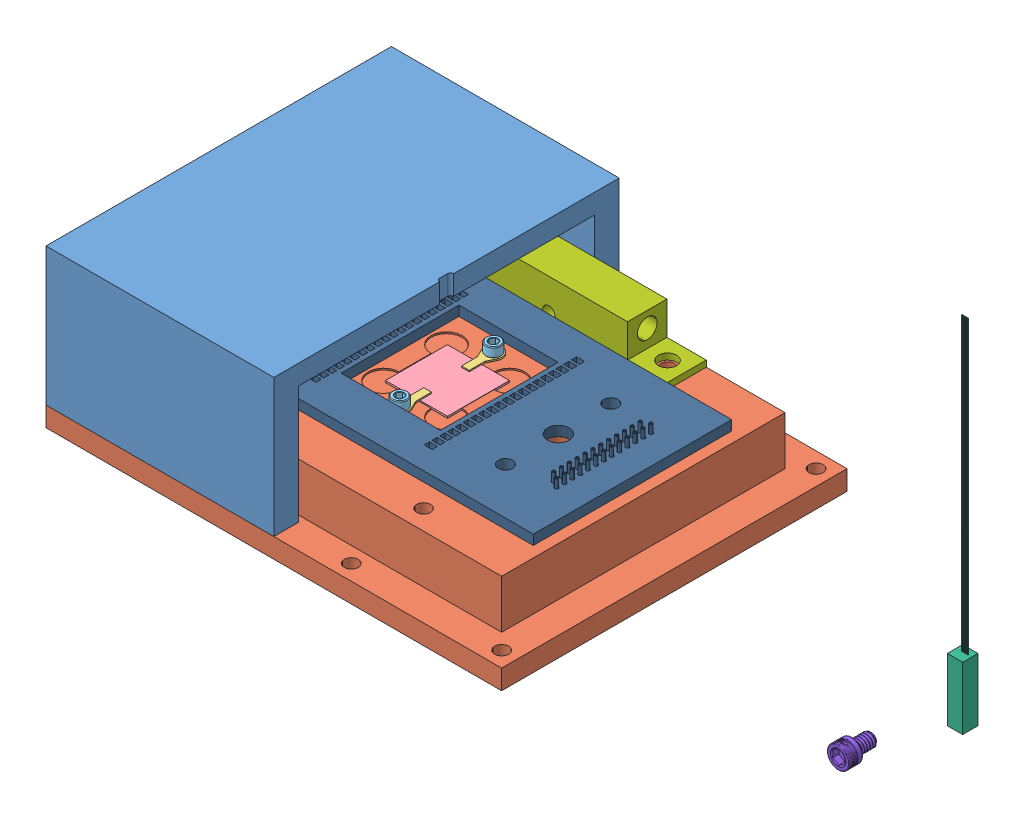
SolidWorks assembly Assembly, configuration Default. Lengths in mm.
Overall size (97.59 65.01 73.15).
14 component instances, 12 part files, 30 mates.
Components (placement in the parent):
- Box-1: Box [Default] at (46.9578 14.8481 6.1828) size (36.75 22.23 55.72)
- Lid-1: Lid [Default] at (10.2078 11.6731 6.1828) size (73.5 11 55.72)
- BeCu_Clamp-1: BeCu_Clamp [Default] at (46.9578 22.6731 26.4812) size (2.82 0.25 5.93)
- example_chip-2: example_chip [Default] at (42.0328 22.4231 28.9678) size (10 0.3 10)
- 92196A047_18-8 Stainless Steel Socket Head Screw-1: 92196A047_18-8 Stainless Steel Socket Head Screw [92196A047] at (46.9578 22.8954 26.4812) x (0.889022 0 -0.457865) z (0 1 0) size (2.44 2.44 3.27)
- 92196A047_18-8 Stainless Steel Socket Head Screw-2: 92196A047_18-8 Stainless Steel Socket Head Screw [92196A047] at (46.9578 22.8954 41.6044) x (0.945947 0 -0.32432) z (0 1 0) size (2.44 2.44 3.27)
- BeCu_Clamp-2: BeCu_Clamp [Default] at (46.9578 22.6731 41.6044) x (-1 0 0) z (0 0 -1) size (2.82 0.25 5.93)
- Fiber_Bundle-2: Fiber_Bundle [Default] at (84.9226 -27.9378 -11.2493) size (2.48 57.1 2.48)
- Heater_Cart_02-1: Heater_Cart_02 [Default] at (34.2578 22.6731 11.1928) x (1 0 0) z (0 1 0) size (38.1 6.35 6.35)
- KM200B-Solidworks_edited-1: KM200B-Solidworks_edited [Default] at (7.5017 57.3012 -5.8381) x (0.999991 0 0.004196) z (0 -1 0) size (77.47 77.47 44.39) (hidden)
- 91251A072_2-56_1_8th_Black-Oxide Alloy Steel Socket Head Screw-1: 91251A072_2-56_1_8th_Black-Oxide Alloy Steel Socket Head Screw [91251A072] at (106.0168 -2.4813 27.2472) size (3.57 3.57 5.6)
- Bottom_Block_off_plate-1: Bottom_Block_off_plate [Default] at (26.9228 9.6731 25.6928) size (40.07 2 16.7)
- micro-d-tes-aaray.step-2: micro-d-tes-aaray.step [Default] at (16.9578 22.6731 50.0428) x (0 0 -1) z (0 1 0) size (32 60 13.01)
- 380-025-213L001.step-1: 380-025-213L001.step [Default] at (18.4828 17.2231 34.0428) x (0 0 -1) z (0 1 0) size (29.7 7.35 10.8)
Mates (geometry in assembly coordinates):
- Coincident1: coincident anti-aligned: plane of Box-1 through (46.9578 14.8481 6.1828) normal (0 -1 0); plane of Lid-1 through (10.2078 14.8481 6.1828) normal (0 1 0)
- Concentric4: concentric aligned: cylinder of Lid-1 through (62.9328 22.6731 14.3678) axis (0 1 0) radius 1.1303; circle of Heater_Cart_02-1
- Concentric5: concentric aligned: circle of Lid-1; circle of Heater_Cart_02-1
- Coincident2: coincident anti-aligned: plane of Lid-1 through (10.2078 22.6731 6.1828) normal (0 1 0); plane of Heater_Cart_02-1 through (34.2578 22.6731 11.1928) normal (0 -1 0)
- Concentric6: concentric anti-aligned: cylinder of BeCu_Clamp-1 through (46.9578 22.9271 26.4812) axis (0 -1 0) radius 0.8382; circle of 92196A047_18-8 Stainless Steel Socket Head Screw-1
- Coincident3: coincident anti-aligned: plane of BeCu_Clamp-1 through (46.9578 22.9271 26.4812) normal (0 1 0); plane of 92196A047_18-8 Stainless Steel Socket Head Screw-1 through (46.3996 22.9271 25.3973) normal (0 -1 0)
- Concentric7: concentric aligned: cylinder of Lid-1 through (46.9578 22.6731 26.4812) axis (0 1 0) radius 0.5956; circle of 92196A047_18-8 Stainless Steel Socket Head Screw-1
- Coincident4: coincident anti-aligned: plane of Lid-1 through (10.2078 22.6731 6.1828) normal (0 1 0); plane of BeCu_Clamp-1 through (46.9578 22.6731 26.4812) normal (0 -1 0)
- Concentric8: concentric aligned: cylinder of 92196A047_18-8 Stainless Steel Socket Head Screw-2 through (46.9578 21.3396 41.6044) axis (0 -1 0) radius 1.2192; cylinder of BeCu_Clamp-2 through (46.9578 22.9271 41.6044) axis (0 -1 0) radius 0.8382
- Coincident5: coincident anti-aligned: plane of 92196A047_18-8 Stainless Steel Socket Head Screw-2 through (46.5624 22.9271 40.4511) normal (0 -1 0); plane of BeCu_Clamp-2 through (46.9578 22.9271 41.6044) normal (0 1 0)
- Concentric9: concentric anti-aligned: cylinder of Lid-1 through (46.9578 22.6731 41.6044) axis (0 1 0) radius 0.5956; cylinder of 92196A047_18-8 Stainless Steel Socket Head Screw-2 through (46.9578 21.3396 41.6044) axis (0 -1 0) radius 1.2192
- Coincident6: coincident anti-aligned: plane of Lid-1 through (10.2078 22.6731 6.1828) normal (0 1 0); plane of BeCu_Clamp-2 through (46.9578 22.6731 41.6044) normal (0 -1 0)
- Parallel1: parallel aligned: plane of BeCu_Clamp-1 through (47.5801 22.9271 26.4812) normal (1 0 0); plane of BeCu_Clamp-2 through (47.5801 22.9271 41.6044) normal (1 0 0)
- Parallel2: parallel anti-aligned: plane of Lid-1 through (52.0328 22.4231 6.1828) normal (-1 0 0); plane of BeCu_Clamp-1 through (47.5801 22.9271 26.4812) normal (1 0 0)
- Concentric10: concentric anti-aligned: cylinder of Lid-1 through (64.9928 22.6731 34.0428) axis (0 -1 0) radius 1.7272; cylinder of KM200B-Solidworks_edited-1 through (64.9928 0.3201 34.0428) axis (0 1 0) radius 1.7272
- Parallel3: parallel anti-aligned: cylinder of Lid-1 through (28.9228 22.6731 34.0428) axis (0 -1 0) radius 1.7272; cylinder of KM200B-Solidworks_edited-1 through (28.9252 0.3201 33.8915) axis (0 1 0) radius 1.7272
- Coincident9: coincident anti-aligned: plane of Lid-1 through (10.2078 11.6731 6.1828) normal (0 -1 0); plane of Bottom_Block_off_plate-1 through (26.9228 11.6731 25.6928) normal (0 1 0)
- Coincident10: coincident anti-aligned: plane of Lid-1 through (52.0328 22.4231 6.1828) normal (-1 0 0); plane of example_chip-2 through (52.0328 22.7231 28.9678) normal (1 0 0)
- Coincident11: coincident anti-aligned: plane of Lid-1 through (10.2078 22.4231 28.9678) normal (0 0 1); plane of example_chip-2 through (42.0328 22.7231 28.9678) normal (0 0 -1)
- Coincident12: coincident anti-aligned: plane of Lid-1 through (41.8828 22.4231 28.9678) normal (0 1 0); plane of example_chip-2 through (42.0328 22.4231 28.9678) normal (0 -1 0)
- Concentric28: concentric aligned: cylinder of Lid-1 through (28.9578 22.6731 25.5428) axis (0 1 0) radius 0.889; cylinder of micro-d-tes-aaray.step-2 through (28.9578 21.8831 25.5428) axis (0 1 0) radius 1.15
- Concentric29: concentric aligned: cylinder of Lid-1 through (28.9578 22.6731 42.5428) axis (0 1 0) radius 0.889; cylinder of micro-d-tes-aaray.step-2 through (28.9578 21.8831 42.5428) axis (0 1 0) radius 1.15
- Coincident19: coincident anti-aligned: plane of Lid-1 through (10.2078 22.6731 6.1828) normal (0 1 0); plane of micro-d-tes-aaray.step-2 through (46.9578 22.6731 34.0428) normal (0 -1 0)
- Parallel5: parallel anti-aligned: plane of micro-d-tes-aaray.step-2 through (25.8238 17.2231 18.7548) normal (0 -1 0); plane of 380-025-213L001.step-1 through (25.8238 12.3231 49.3308) normal (0 1 0)
- Concentric31: concentric aligned: cylinder of micro-d-tes-aaray.step-2 through (21.6078 16.3231 41.6628) axis (0 -1 0) radius 0.475; cylinder of 380-025-213L001.step-1 through (21.6078 15.8227 41.6628) axis (0 -1 0) radius 0.285
- Concentric32: concentric aligned: cylinder of micro-d-tes-aaray.step-2 through (21.6078 16.3231 26.4228) axis (0 -1 0) radius 0.475; cylinder of 380-025-213L001.step-1 through (21.6078 15.8227 26.4228) axis (0 -1 0) radius 0.285
- Coincident21: coincident: plane of micro-d-tes-aaray.step-2 through (25.8238 17.2231 18.7548) normal (0 -1 0); line of 380-025-213L001.step-1 through (19.5528 17.2231 42.1928) axis (0 0 -1)
- Concentric33: concentric aligned: cylinder of Lid-1 through (28.9228 11.6731 40.3928) axis (0 -1 0) radius 0.889; cylinder of Bottom_Block_off_plate-1 through (28.9228 11.6731 40.3928) axis (0 -1 0) radius 1.1303
- Concentric34: concentric aligned: cylinder of Lid-1 through (64.9928 11.6731 27.6928) axis (0 -1 0) radius 0.889; cylinder of Bottom_Block_off_plate-1 through (64.9928 11.6731 27.6928) axis (0 -1 0) radius 1.1303
- Concentric35: concentric anti-aligned: cylinder of Box-1 through (12.7078 14.8481 59.4028) axis (0 -1 0) radius 0.889; cylinder of Lid-1 through (12.7078 14.8481 59.4028) axis (0 1 0) radius 1.1303
